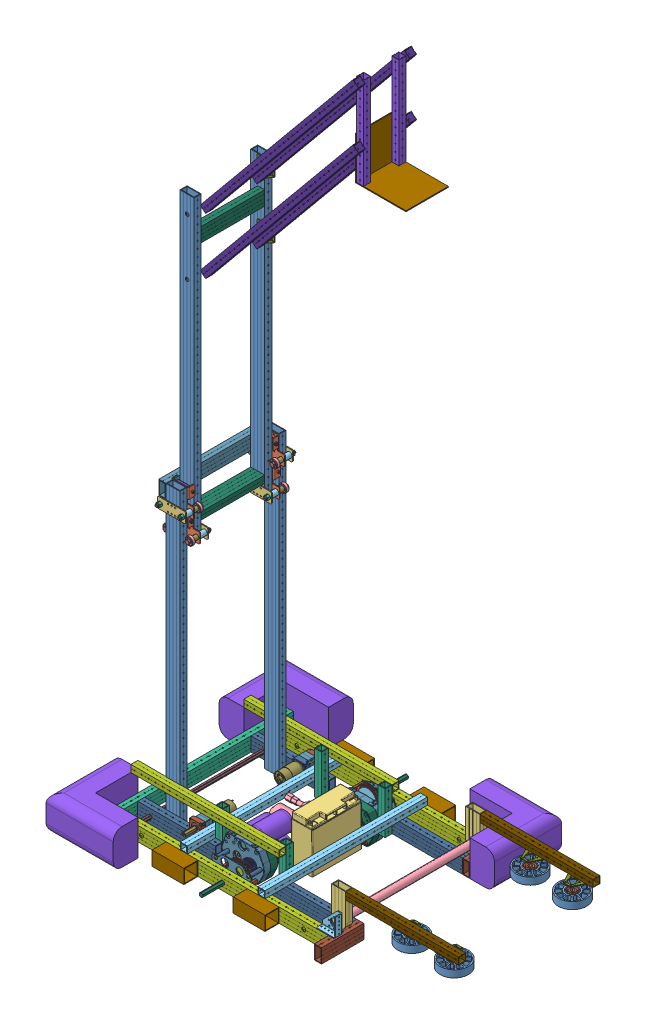
SolidWorks assembly Test Robot 2, configuration Default. Lengths in mm. (continued)
Components (placement in the parent): (continued)
- Test Base 2-1: Test Base 2 [Default] at (327.6786 481.923 -175.606) size (990.6 253.34 863.6) (continued)
  - 3 CIM Ball Shifter with WCD Output-2: 3 CIM Ball Shifter with WCD Output [Default] at (711.3612 320.9643 338.8075) x (0 -1 0) z (0 0 -1) size (169.11 183.68 312.65) (continued)
    - Nylock Nut_NNY2520-ZC-2: Nylock Nut_NNY2520-ZC [Default] at (48.8823 -3.175 37.846) x (0 0 -1) z (-1 0 0) size (12.85 11.89 7.62)
    - Nylock Nut_NNY2520-ZC-3: Nylock Nut_NNY2520-ZC [Default] at (44.45 85.725 7.8613) x (0 1 0) z (0 0 -1) size (12.85 11.89 7.62)
    - 276-1027-001-1: 276-1027-001 [Default] at (47.625 58.1787 6.35) x (0 1 0) z (-1 0 0) size (8.61 5.64 9.94)
    - 276-1027-001-2: 276-1027-001 [Default] at (-47.625 58.1787 6.35) x (0 -1 0) z (1 0 0) size (8.61 5.64 9.94)
    - SCREW-832-1750-1: SCREW-832-1750 [Default] at (-47.625 58.1787 47.0408) x (0 0 -1) z (-0.960822 -0.277167 0) size (46.66 7.92 7.92)
    - SCREW-832-1750-2: SCREW-832-1750 [Default] at (47.625 58.1787 47.0408) x (0 0 -1) z (-0.960822 -0.277167 0) size (46.66 7.92 7.92)
    - Nylock Nut_NNY2520-ZC-4: Nylock Nut_NNY2520-ZC [Default] at (44.45 -15.875 7.8613) x (0 1 0) z (0 0 -1) size (12.85 11.89 7.62)
    - 217-2428-004 Rev3-1: 217-2428-004 Rev3 [Default] at (0 53.4162 22.7711) x (-0.709585 0.70462 0) z (0 0 1) size (11 9.53 43.92)
    - SBS1_SBS-2520-1625SS-1: SBS1_SBS-2520-1625SS [Default] at (44.45 85.725 42.4688) x (0 0 -1) z (-0.251219 0.96793 0) size (45.3 11.2 11.18)
    - SBS1_SBS-2520-1625SS-2: SBS1_SBS-2520-1625SS [Default] at (44.45 -15.875 42.4688) x (0 0 -1) z (-0.251219 0.96793 0) size (45.3 11.2 11.18)
    - SBS1_SBS2520-1750-1: SBS1_SBS2520-1750 [Default] at (-44.45 85.725 7.4422) x (0 0 1) z (-0.031478 0.999504 0) size (48.48 11.22 11.17)
    - SBS1_SBS2520-1750-2: SBS1_SBS2520-1750 [Default] at (-44.45 -15.875 7.4422) x (0 0 1) z (-0.937114 -0.349025 0) size (48.48 11.22 11.17)
    - 217-2428-021 Rev1-1: 217-2428-021 Rev1 [Default] at (0 53.4162 9.5123) x (0.451333 -0.892356 0) z (0 0 1) size (15.88 15.88 3.17)
    - 217-2428-029 Rev1-1: 217-2428-029 Rev1 [Default] at (0 53.4162 36.957) x (0.999846 0.017557 0) z (0 0 1) size (15.88 15.88 1.12)
    - Grayhill Lock Washer-1: Grayhill Lock Washer [Default] at (12.7 -21.997 -18.6817) x (0.467173 -0.884166 0) z (0 0 1) size (19.69 19.69 0.74)
    - Grayhill Nut-1: Grayhill Nut [Default] at (12.7 -21.997 -17.0434) x (0.984088 0.177684 0) z (0 0 1) size (18.33 15.88 2.54)
    - 217-2000-1: 217-2000 [Default] at (0 92.8624 0) x (0 0 -1) z (0.223996 -0.97459 0) size (150.2 64.01 64.01)
    - 217-2000-2: 217-2000 [Default] at (-36.9798 39.6868 0) x (0 0 -1) z (0.996195 -0.087156 0) size (150.2 64.01 64.01)
    - 217-2000-3: 217-2000 [Default] at (36.9798 39.6868 0) x (0 0 -1) z (0.996195 0.087156 0) size (150.2 64.01 64.01)
    - Grahill Encoder-1: Grahill Encoder [Default] at (12.7 -21.997 -16.1798) x (-0.580071 0.814566 0) z (-0.814566 -0.580071 0) size (31.75 31.12 31.75)
    - 217-3195-009 Rev1_wcd 2-1: 217-3195-009 Rev1_wcd 2 [Default] at (0 85.725 50.546) x (-0.998427 -0.056065 0) z (0 0 1) size (12.7 12.7 41.27)
    - 217-3195-006 Rev1_WCD-1: 217-3195-006 Rev1_WCD [Default] at (-44.45 85.725 44.1452) x (0.5 0.866025 0) z (0 0 1) size (12.7 14.66 47.62)
    - 217-3195-009 Rev1_wcd 2-2: 217-3195-009 Rev1_wcd 2 [Default] at (0 -31.75 50.546) x (0.947633 0.319361 0) z (0 0 1) size (12.7 12.7 41.27)
    - 217-3195-006 Rev1_WCD-2: 217-3195-006 Rev1_WCD [Default] at (-44.45 -15.875 44.1452) x (0.5 -0.866025 0) z (0 0 1) size (12.7 14.66 47.62)
    - Nylock Nut_NNY2520-ZC-5: Nylock Nut_NNY2520-ZC [Default] at (0 -31.75 45.0723) x (-0.5 0.866025 0) z (0 0 -1) size (12.85 11.89 7.62)
    - Nylock Nut_NNY2520-ZC-6: Nylock Nut_NNY2520-ZC [Default] at (0 85.725 45.0723) x (-0.5 0.866025 0) z (0 0 -1) size (12.85 11.89 7.62)
    - SBS1_SBS-2520-2250-1: SBS1_SBS-2520-2250 [Default] at (0 -31.75 98.298) x (0 0 -1) z (-0.933488 -0.358607 0) size (61.18 11.22 11.17)
    - SBS1_SBS2520-0625ZC-1: SBS1_SBS2520-0625ZC [Default] at (-44.45 85.725 98.298) x (0 0 -1) z (0.400817 0.916158 0) size (19.57 11.22 11.17)
    - SBS1_SBS2520-0625ZC-2: SBS1_SBS2520-0625ZC [Default] at (-44.45 -15.875 98.298) x (0 0 -1) z (-0.75178 -0.659414 0) size (19.57 11.22 11.17)
    - SBS1_SBS-2520-2250-2: SBS1_SBS-2520-2250 [Default] at (0 85.725 98.298) x (0 0 -1) z (0.056677 -0.998393 0) size (61.18 11.22 11.17)
    - 217-3195-003 rev2-1: 217-3195-003 rev2 [Default] at (0 0 94.9452) size (88.62 139.7 3.17)
    - 217-2617-003 Rev1-1: 217-2617-003 Rev1 [Default] at (-39.878 35.5392 121.8535) x (-0.5 -0.866025 0) z (0 0 1) size (14.66 12.7 152.4)
    - 217-3109-001 Rev1-1: 217-3109-001 Rev1 [Default] at (-39.878 35.5392 49.1808) x (0 0 1) z (0.312889 -0.94979 0) size (7.94 28.57 28.57)
    - 217-2734-001 Rev3-1: 217-2734-001 Rev3 [Default] at (-39.878 35.5392 98.1202) x (1 0 0) z (0 1 0) size (31.12 7.94 31.12)
    - 217-2617-004 Rev1_97431A340_grv-1: 217-2617-004 Rev1_97431A340_grv [Default] at (-39.878 35.5392 54.8961) x (0 0 1) z (-0.124043 -0.992277 0) size (1.07 20.42 18.58)
    - 217-2617-004 Rev1_97431A340_grv-2: 217-2617-004 Rev1_97431A340_grv [Default] at (0 0 69.215) x (0 0 1) z (-0.124043 -0.992277 0) size (1.07 20.42 18.58)
    - 217-2702-001_20t-1: 217-2702-001_20t [Default] at (0 0 62.357) x (0.998435 0.055929 0) z (0 0 1) size (28.2 28.2 12.65)
    - 217-2715-002 Rev1_64t-1: 217-2715-002 Rev1_64t [Default] at (-39.878 35.5392 61.7541) x (0.866025 -0.5 0) z (0 0 1) size (84.3 84.3 12.65)
    - 217-2704-001_24-1: 217-2704-001_24 [Default] at (0 0 62.357) x (0.450781 0.892635 0) z (0 0 -1) size (33.29 33.29 12.65)
    - 217-2714-002 Rev1_60t-1: 217-2714-002 Rev1_60t [Default] at (-39.878 35.5392 61.7541) x (0.866025 -0.5 0) z (0 0 1) size (78.95 78.95 12.65)
    - 217-3221-002 Rev1-1: 217-3221-002 Rev1 [Default] at (-39.878 35.5392 61.7414) x (0 -1 0) z (0 0 1) size (71.39 71.45 12.62)
    - 217-2705-001_30t-1: 217-2705-001_30t [Default] at (0 0 62.357) x (0.547654 -0.836705 0) z (0 0 1) size (41.01 41.12 12.65)
    - 217-2712-002 Rev1_50t-1: 217-2712-002 Rev1_50t [Default] at (-39.878 35.5392 61.7541) x (0.866025 -0.5 0) z (0 0 1) size (66.7 66.76 12.65)
    - 217-2706-001_34t-1: 217-2706-001_34t [Default] at (0 0 62.357) x (0.998435 0.055929 0) z (0 0 1) size (46.46 46.56 12.65)
    - 217-3288-001 Rev3-1: 217-3288-001 Rev3 [Default] at (0 0 0.0889) x (0.055929 -0.998435 0) z (0 0 1) size (99.51 99.53 98.3)
      - 217-2428-008 Rev2-1: 217-2428-008 Rev2 [Default] at (0 0 10.2679) size (31.75 31.75 1.59)
      - 217-2428-028 Rev1_97633A250-1: 217-2428-028 Rev1_97633A250 [Default] at (0 0 37.1221) x (0 0 1) z (0.9357 -0.352797 0) size (1.07 23.39 21.18)
      - 217-4099-000 Rev2_high gear-1: 217-4099-000 Rev2_high gear [Default] x (-1 0 0) z (0 0 1) size (22.23 22.23 98.3)
        - 217-4098-005 Rev1_91612A226-1: 217-4098-005 Rev1_91612A226 [Default] at (0 0 46.2661) x (-0.144757 0 0.989467) z (0 -1 0) size (3.02 3.15 18.22)
        - 217-4098-003 Rev2-1: 217-4098-003 Rev2 [Default] x (1 0 0) z (0 0 -1) size (22.23 22.23 55.94)
        - 217-4099-002 Rev3-1: 217-4099-002 Rev3 [Default] at (0 0 53.467) x (0 0 1) z (-1 0 0) size (40.96 12.73 14.67)
        - 217-4098-004 Rev1-1: 217-4098-004 Rev1 [Default] at (0 0 14.2494) x (0.393904 0.919152 0) z (0 0 1) size (11.68 11.68 56)
      - 217-2428-007 Rev1-1: 217-2428-007 Rev1 [Default] at (7.809 4.5085 14.2494) x (-0.69071 0.455693 -0.561483) z (-0.67559 -0.683536 0.276329) size (6.35 6.35 6.35)
      - 217-2428-007 Rev1-2: 217-2428-007 Rev1 [Default] at (5.4343 3.1375 26.9494) x (-0.162331 -0.978398 0.128005) z (0.857281 -0.204076 -0.472676) size (6.35 6.35 6.35)
      - 217-3212-101 Rev1-1: 217-3212-101 Rev1 [Default] at (-11.5751 10.4131 45.3224) x (0.923728 0.383049 0) z (0 0 -1) size (46.46 46.56 12.7)
        - 217-2428-022 Rev1-1: 217-2428-022 Rev1 [Default] at (6.7035 14.0527 24.6087) size (28.57 28.57 6.1)
        - 217-3212-001 Rev1_34t-1: 217-3212-001 Rev1_34t [Default] at (6.7035 14.0527 27.9107) size (46.46 46.56 11.11)
      - 217-3222-101 Rev1-1: 217-3222-101 Rev1 [Default] at (21.0941 -5.2804 52.7371) x (-0.889163 -0.457591 0) z (0 0 -1) size (73.87 73.92 12.7)
        - 217-2428-022 Rev1-1: 217-2428-022 Rev1 [Default] at (16.3398 14.3476 19.3234) size (28.57 28.57 6.1)
        - 217-3222-001 Rev1_Spur01-1: 217-3222-001 Rev1_Spur01 [Default] at (16.3398 14.3476 22.6254) x (0.999377 0.0353 0) z (0 0 1) size (71.39 71.45 11.11)
      - 217-2428-007 Rev1-3: 217-2428-007 Rev1 [Default] at (-5.4343 3.1375 26.9494) x (0.928483 0.348617 0.128005) z (-0.251905 0.844465 -0.472676) size (6.35 6.35 6.35)
      - 217-2428-007 Rev1-4: 217-2428-007 Rev1 [Default] at (0 -6.275 26.9494) x (-0.766153 0.629782 0.128005) z (-0.605376 -0.640389 -0.472676) size (6.35 6.35 6.35)
      - 217-2428-007 Rev1-5: 217-2428-007 Rev1 [Default] at (-7.809 4.5085 14.2494) x (-0.049287 -0.826019 -0.561483) z (0.929754 -0.24331 0.276329) size (6.35 6.35 6.35)
      - 217-2428-007 Rev1-6: 217-2428-007 Rev1 [Default] at (0 -9.017 14.2494) x (0.739997 0.370326 -0.561483) z (-0.254164 0.926846 0.276329) size (6.35 6.35 6.35)
    - 217-3210-001 Rev1_30t-1: 217-3210-001 Rev1_30t [Default] at (0 53.4162 30.0736) x (-0.966828 0.255427 0) z (0 0 1) size (41.01 41.12 12.65)
    - 217-2711-002 Rev1_50t-1: 217-2711-002 Rev1_50t [Default] at (0 53.4162 17.4244) x (0.262208 -0.965011 0) z (0 0 1) size (66.7 66.76 12.65)
  - Base Front Rail-2: Base Front Rail [Default] at (1069.5219 360.9185 -429.2377) size (25.4 50.8 152.4)
  - Blue Bumper-3: Blue Bumper [Default] at (180.5219 335.5185 942.3623) size (241.3 127 241.3)
  - Blue Bumper-4: Blue Bumper [Default] at (180.5219 335.5185 78.7623) x (0 0 1) z (-1 0 0) size (241.3 127 241.3)
  - Battery_12V-1: Battery_12V [Default] at (781.3061 335.5185 454.7754) x (0 0 1) z (0 1 0) size (177.8 76.2 167.13)
  - Compressor_90C-1: Compressor_90C [Default] at (627.7537 373.1105 499.1323) x (0 0 -1) z (1 0 0) size (53.59 121.98 156.21)
  - Base Side Rail Internal-5: Base Side Rail Internal [Default] at (307.5219 360.9185 307.3623) x (0 0 -1) z (1 0 0) size (25.4 50.8 279.4)
  - Base Side Rail Internal-6: Base Side Rail Internal [Default] at (307.5219 360.9185 713.7623) x (0 0 -1) z (1 0 0) size (25.4 50.8 279.4)
  - Superstructure Lower Crossbar-1: Superstructure Lower Crossbar [Default] at (815.5219 399.0185 53.3623) size (25.4 25.4 584.2)
  - Superstructure Upright-1: Superstructure Upright [Default] at (790.1219 1084.8185 688.3623) x (1 0 0) z (0 -1 0) size (25.4 25.4 152.4)
  - Superstructure Upright-2: Superstructure Upright [Default] at (790.1219 1084.8185 332.7623) x (1 0 0) z (0 -1 0) size (25.4 25.4 152.4)
  - Superstructure Upright-3: Superstructure Upright [Default] at (561.5219 1084.8185 332.7623) x (1 0 0) z (0 -1 0) size (25.4 25.4 152.4)
  - Superstructure Upright-4: Superstructure Upright [Default] at (561.5219 1084.8185 689.3363) x (1 0 0) z (0 -1 0) size (25.4 25.4 152.4)
  - Superstructure Lower Crossbar-2: Superstructure Lower Crossbar [Default] at (536.1219 399.0185 53.3623) size (25.4 25.4 584.2)
  - Superstructure Crossbar-1: Superstructure Crossbar [Default] at (53.5219 475.2185 713.7623) x (0 0 -1) z (1 0 0) size (25.4 25.4 533.4)
  - Superstructure Crossbar-2: Superstructure Crossbar [Default] at (53.5219 475.2185 307.3623) x (0 0 -1) z (1 0 0) size (25.4 25.4 533.4)
- PowerUp Cube-3: PowerUp Cube [Default] at (1484.2166 1060.7016 182.5563) x (1 0 0) z (0 0 -1) size (330.2 279.4 330.2) (hidden)
- Intake Mechansim-1: Intake Mechansim [Default] at (1364.1836 3104.9251 338.871) x (-1 0 0) z (0 1 0) size (25.4 25.4 330.2)
  - Elevator Top Crossbar-1: Elevator Top Crossbar [Default] at (81.2508 124.0592 -460.6133) size (25.4 25.4 330.2) (hidden)
- PowerUp Cube-4: PowerUp Cube [Default] at (1295.6328 3203.1118 170.8303) x (1 0 0) z (0 0 -1) size (330.2 279.4 330.2) (hidden)
- VersaFrame Corner Gusset-2: VersaFrame Corner Gusset [Default] at (1409.9006 868.2415 601.6563) x (0 1 0) z (0 0 1) size (69.72 69.72 25.4)
- Top Bottom Grasper-1: Top Bottom Grasper [Default] at (1103.9738 3449.2709 552.0299) x (0 0 -1) z (0 -1 0) size (152.4 180.97 333.38)
  - Elevator Top Crossbar-1: Elevator Top Crossbar [Default] at (152.5996 178.9591 -350.7409) size (25.4 25.4 330.2)
  - Elevator Top Crossbar-2: Elevator Top Crossbar [Default] at (279.5996 178.9591 -350.7409) size (25.4 25.4 330.2)
  - Cube Intake Bottom Support-1: Cube Intake Bottom Support [Default] at (139.8996 163.0841 246.1591) x (0 1 0) z (1 0 0) size (180.97 155.57 152.4)
- 217-2 Stage Versaplanetary STEP-1: 217-2 Stage Versaplanetary STEP [Default] at (830.1006 889.2415 170.5813) size (44.3 44.3 179.1)
  - 217-2625-001 Rev1-1: 217-2625-001 Rev1 [Default] at origin size (42 42 18)
  - 217-2625-002 Rev1-1: 217-2625-002 Rev1 [Default] at (0 0 -29.4) size (42 42 17.13)
  - 217-2625-003 Rev1-1: 217-2625-003 Rev1 [Default] at (0 0 -43.6478) x (1 0 0) z (0 0 -1) size (17 17 64.12)
  - 217-2625-009 Rev1-1: 217-2625-009 Rev1 [Default] at (0 0 -3.48) x (0 -1 0) z (0 0 -1) size (18 18 13)
  - 217-2816-001 Rev1-1: 217-2816-001 Rev1 [Default] at (0 0 -16.85) x (1 0 0) z (0 0 -1) size (42 42 14.5)
  - 217-2625-007 Rev1_Sun_Driver01-1: 217-2625-007 Rev1_Sun_Driver01 [Default] at (0 0 -11.767) x (0.055822 0.998441 0) z (0 0 1) size (14.49 14.49 12.72)
  - 217-2625-100-1: 217-2625-100 [Default] at (0 0 -18.467) x (0 1 0) z (0 0 1) size (39.26 38.9 12.7)
    - 217-2625-008 Rev1-1: 217-2625-008 Rev1 [Default] at origin size (34.7 34.7 4.7)
    - 217-2625-010 Rev1-1: 217-2625-010 Rev1 [Default] at (0 10.193 3.65) x (0.999813 0.019336 0) z (0 0 1) size (4 4 12)
    - 217-2625-010 Rev1-2: 217-2625-010 Rev1 [Default] at (8.691 -5.3258 3.65) size (4 4 12)
    - 217-2625-010 Rev1-3: 217-2625-010 Rev1 [Default] at (-8.691 -5.3258 3.65) size (4 4 12)
    - 217-2625-005 Rev1_Planet_Revolving_Follower01-1: 217-2625-005 Rev1_Planet_Revolving_Follower01 [Default] at (8.691 -5.3258 6.35) x (0.932816 0.360354 0) z (0 0 1) size (16.91 16.92 8)
    - 217-2625-005 Rev1_Planet_Revolving_Follower01-2: 217-2625-005 Rev1_Planet_Revolving_Follower01 [Default] at (-8.691 -5.3258 6.35) x (-0.932788 -0.360426 0) z (0 0 1) size (16.91 16.92 8)
    - 217-2625-005 Rev1_Planet_Revolving_Follower01-3: 217-2625-005 Rev1_Planet_Revolving_Follower01 [Default] at (0 10.193 6.35) x (0.893583 0.448898 0) z (0 0 1) size (16.91 16.92 8)
  - 217-2822-003 Rev4-1: 217-2822-003 Rev4 [Default] at (0 0 9) x (0 1 0) z (0 0 1) size (42 42 4.8)
  - 217-2625-011 Rev1-1: 217-2625-011 Rev1 [Default] at (0 0 1.37) x (1 0 0) z (0 -1 0) size (8.01 7.5 7.94)
  - SSA_SSA0832-0500ZC-1: SSA_SSA0832-0500ZC [Default] at (17.5 -17.5 10.5) x (0.189399 -0.9819 0) z (-0.9819 -0.189399 0) size (6.73 16.76 6.73)
  - 217-2742-1: 217-2742 [Default] at (0 0 -43.1002) x (0 0 1) z (-1 0 0) size (7 28 28)
  - 217-2742-2: 217-2742 [Default] at (0 0 -51.4002) x (0 0 1) z (-0.997393 0.072165 0) size (7 28 28)
  - SSA_SSA0832-1750ZC-1: SSA_SSA0832-1750ZC [Default] at (17.5 -17.5 -47.261) x (1 0 0) z (0 1 0) size (6.73 48.51 6.73)
  - SSA_SSA0832-1750ZC-2: SSA_SSA0832-1750ZC [Default] at (-17.5 17.5 -47.261) x (1 0 0) z (0 1 0) size (6.73 48.51 6.73)
  - 217-2625-018 Rev1_98541A410-1: 217-2625-018 Rev1_98541A410 [Default] at (0 0 -35.4954) x (0 0 -1) z (0.980859 -0.194721 0) size (1 19.6 17.4)
  - 217-2625-017 Rev1_9714K61-1: 217-2625-017 Rev1_9714K61 [Default] at (0 0 -44.1002) x (-0.695225 0.718792 0) z (-0.718792 -0.695225 0) size (28.51 4.98 30.18)
  - PINL-M020-006-S-1: PINL-M020-006-S [Default] at (-18.5 13.6657 -9.5) x (0 0 -1) z (1 0 0) size (6 2 2)
  - PINL-M020-006-S-2: PINL-M020-006-S [Default] at (-18.5 13.6657 -22.2) x (0 0 -1) z (0.23951 -0.970894 0) size (6 2 2)
  - 217-2816-001 Rev1-2: 217-2816-001 Rev1 [Default] at (0 0 -29.55) x (1 0 0) z (0 0 -1) size (42 42 14.5)
  - 217-3106-000 Rev2_NO SUN-1: 217-3106-000 Rev2_NO SUN [Default] at (0 0 -31.5454) size (40.34 37.58 17.71)
    - 217-3106-002 Rev1_Planet_Revolving_Follower01-1: 217-3106-002 Rev1_Planet_Revolving_Follower01 [Default] at (0 10.2965 6.35) x (0.979503 -0.20143 0) z (0 0 1) size (16.8 16.83 8)
    - 217-3106-003 Rev1-1: 217-3106-003 Rev1 [Default] at origin size (34.7 34.7 4.7)
    - 217-3106-001 Rev1_Sun_Driver01-1: 217-3106-001 Rev1_Sun_Driver01 [Default] at (0 0 9.0125) x (1 0 0) z (0 0 -1) size (14.56 14.56 12.7)
    - 217-3106-002 Rev1_Planet_Revolving_Follower01-2: 217-3106-002 Rev1_Planet_Revolving_Follower01 [Default] at (8.917 -5.1482 6.35) x (-0.664195 -0.74756 0) z (0 0 1) size (16.8 16.83 8)
    - 217-3106-002 Rev1_Planet_Revolving_Follower01-3: 217-3106-002 Rev1_Planet_Revolving_Follower01 [Default] at (-8.917 -5.1482 6.35) x (-0.315308 0.948989 0) z (0 0 1) size (16.8 16.83 8)
    - 217-2625-010 Rev1-1: 217-2625-010 Rev1 [Default] at (8.917 -5.1482 3.65) x (0.999617 0.027658 0) z (0 0 1) size (4 4 12)
    - 217-2625-010 Rev1-2: 217-2625-010 Rev1 [Default] at (-8.917 -5.1482 3.65) x (-0.475856 -0.879523 0) z (0 0 1) size (4 4 12)
    - 217-2625-010 Rev1-3: 217-2625-010 Rev1 [Default] at (0 10.2965 3.65) x (-0.523761 0.851865 0) z (0 0 1) size (4 4 12)
  - 775 pro-1: 775 pro [Default] at (0 0 10.5) x (0 0 1) z (-1 0 0) size (88 44.3 44.3)
- 217-2 Stage Versaplanetary STEP-2: 217-2 Stage Versaplanetary STEP [Default] at (830.1006 889.2415 500.3053) x (-1 0 0) z (0 0 -1) size (44.3 44.3 179.1)
  - 217-2625-001 Rev1-1: 217-2625-001 Rev1 [Default] at origin size (42 42 18)
  - 217-2625-002 Rev1-1: 217-2625-002 Rev1 [Default] at (0 0 -29.4) size (42 42 17.13)
  - 217-2625-003 Rev1-1: 217-2625-003 Rev1 [Default] at (0 0 -43.6478) x (1 0 0) z (0 0 -1) size (17 17 64.12)
  - 217-2625-009 Rev1-1: 217-2625-009 Rev1 [Default] at (0 0 -3.48) x (0 -1 0) z (0 0 -1) size (18 18 13)
  - 217-2816-001 Rev1-1: 217-2816-001 Rev1 [Default] at (0 0 -16.85) x (1 0 0) z (0 0 -1) size (42 42 14.5)
  - 217-2625-007 Rev1_Sun_Driver01-1: 217-2625-007 Rev1_Sun_Driver01 [Default] at (0 0 -11.767) x (0.055822 0.998441 0) z (0 0 1) size (14.49 14.49 12.72)
  - 217-2625-100-1: 217-2625-100 [Default] at (0 0 -18.467) x (0 1 0) z (0 0 1) size (39.26 38.9 12.7)
    - 217-2625-008 Rev1-1: 217-2625-008 Rev1 [Default] at origin size (34.7 34.7 4.7)
    - 217-2625-010 Rev1-1: 217-2625-010 Rev1 [Default] at (0 10.193 3.65) x (0.999813 0.019336 0) z (0 0 1) size (4 4 12)
    - 217-2625-010 Rev1-2: 217-2625-010 Rev1 [Default] at (8.691 -5.3258 3.65) size (4 4 12)
    - 217-2625-010 Rev1-3: 217-2625-010 Rev1 [Default] at (-8.691 -5.3258 3.65) size (4 4 12)
    - 217-2625-005 Rev1_Planet_Revolving_Follower01-1: 217-2625-005 Rev1_Planet_Revolving_Follower01 [Default] at (8.691 -5.3258 6.35) x (0.932816 0.360354 0) z (0 0 1) size (16.91 16.92 8)
    - 217-2625-005 Rev1_Planet_Revolving_Follower01-2: 217-2625-005 Rev1_Planet_Revolving_Follower01 [Default] at (-8.691 -5.3258 6.35) x (-0.932788 -0.360426 0) z (0 0 1) size (16.91 16.92 8)
    - 217-2625-005 Rev1_Planet_Revolving_Follower01-3: 217-2625-005 Rev1_Planet_Revolving_Follower01 [Default] at (0 10.193 6.35) x (0.893583 0.448898 0) z (0 0 1) size (16.91 16.92 8)
  - 217-2822-003 Rev4-1: 217-2822-003 Rev4 [Default] at (0 0 9) x (0 1 0) z (0 0 1) size (42 42 4.8)
  - 217-2625-011 Rev1-1: 217-2625-011 Rev1 [Default] at (0 0 1.37) x (1 0 0) z (0 -1 0) size (8.01 7.5 7.94)
  - SSA_SSA0832-0500ZC-1: SSA_SSA0832-0500ZC [Default] at (17.5 -17.5 10.5) x (0.189399 -0.9819 0) z (-0.9819 -0.189399 0) size (6.73 16.76 6.73)
  - 217-2742-1: 217-2742 [Default] at (0 0 -43.1002) x (0 0 1) z (-1 0 0) size (7 28 28)
  - 217-2742-2: 217-2742 [Default] at (0 0 -51.4002) x (0 0 1) z (-0.997393 0.072165 0) size (7 28 28)
  - SSA_SSA0832-1750ZC-1: SSA_SSA0832-1750ZC [Default] at (17.5 -17.5 -47.261) x (1 0 0) z (0 1 0) size (6.73 48.51 6.73)
  - SSA_SSA0832-1750ZC-2: SSA_SSA0832-1750ZC [Default] at (-17.5 17.5 -47.261) x (1 0 0) z (0 1 0) size (6.73 48.51 6.73)
  - 217-2625-018 Rev1_98541A410-1: 217-2625-018 Rev1_98541A410 [Default] at (0 0 -35.4954) x (0 0 -1) z (0.980859 -0.194721 0) size (1 19.6 17.4)
  - 217-2625-017 Rev1_9714K61-1: 217-2625-017 Rev1_9714K61 [Default] at (0 0 -44.1002) x (-0.695225 0.718792 0) z (-0.718792 -0.695225 0) size (28.51 4.98 30.18)
  - PINL-M020-006-S-1: PINL-M020-006-S [Default] at (-18.5 13.6657 -9.5) x (0 0 -1) z (1 0 0) size (6 2 2)
  - PINL-M020-006-S-2: PINL-M020-006-S [Default] at (-18.5 13.6657 -22.2) x (0 0 -1) z (0.23951 -0.970894 0) size (6 2 2)
  - 217-2816-001 Rev1-2: 217-2816-001 Rev1 [Default] at (0 0 -29.55) x (1 0 0) z (0 0 -1) size (42 42 14.5)
  - 217-3106-000 Rev2_NO SUN-1: 217-3106-000 Rev2_NO SUN [Default] at (0 0 -31.5454) size (40.34 37.58 17.71)
    - 217-3106-002 Rev1_Planet_Revolving_Follower01-1: 217-3106-002 Rev1_Planet_Revolving_Follower01 [Default] at (0 10.2965 6.35) x (0.979503 -0.20143 0) z (0 0 1) size (16.8 16.83 8)
    - 217-3106-003 Rev1-1: 217-3106-003 Rev1 [Default] at origin size (34.7 34.7 4.7)
    - 217-3106-001 Rev1_Sun_Driver01-1: 217-3106-001 Rev1_Sun_Driver01 [Default] at (0 0 9.0125) x (1 0 0) z (0 0 -1) size (14.56 14.56 12.7)
    - 217-3106-002 Rev1_Planet_Revolving_Follower01-2: 217-3106-002 Rev1_Planet_Revolving_Follower01 [Default] at (8.917 -5.1482 6.35) x (-0.664195 -0.74756 0) z (0 0 1) size (16.8 16.83 8)
    - 217-3106-002 Rev1_Planet_Revolving_Follower01-3: 217-3106-002 Rev1_Planet_Revolving_Follower01 [Default] at (-8.917 -5.1482 6.35) x (-0.315308 0.948989 0) z (0 0 1) size (16.8 16.83 8)
    - 217-2625-010 Rev1-1: 217-2625-010 Rev1 [Default] at (8.917 -5.1482 3.65) x (0.999617 0.027658 0) z (0 0 1) size (4 4 12)
    - 217-2625-010 Rev1-2: 217-2625-010 Rev1 [Default] at (-8.917 -5.1482 3.65) x (-0.475856 -0.879523 0) z (0 0 1) size (4 4 12)
    - 217-2625-010 Rev1-3: 217-2625-010 Rev1 [Default] at (0 10.2965 3.65) x (-0.523761 0.851865 0) z (0 0 1) size (4 4 12)
  - 775 pro-1: 775 pro [Default] at (0 0 10.5) x (0 0 1) z (-1 0 0) size (88 44.3 44.3)
- Elevator Hex Shaft-1: Elevator Hex Shaft [Default] at (667.4706 842.8161 144.4563) size (13.74 12.75 533.4)
Mates (geometry in assembly coordinates):
- Distance6: distance = 25.4 mm anti-aligned: plane of Elevator Moving Stage-1/Elevator Fixed Frame-1 through (749.5006 2773.2415 196.2303) normal (0 0 -1); plane of Elevator Base Frame-1/Elevator Fixed Frame-2 through (698.7006 1884.2415 170.8303) normal (0 0 1)
- Coincident11: coincident aligned: plane of Elevator Base Frame-1/Elevator Fixed Frame-1 through (749.5006 1884.2415 501.0303) normal (1 0 0); plane of Elevator Moving Stage-1/Elevator Fixed Frame-2 through (749.5006 2773.2415 475.6303) normal (1 0 0)
- LimitDistance1: limit distance = 889 mm aligned: plane of Elevator Base Frame-1/Elevator Fixed Frame-1 through (724.1006 1884.2415 513.7303) normal (0 1 0); plane of Elevator Moving Stage-1/Elevator Fixed Frame-2 through (724.1006 2773.2415 462.9303) normal (0 1 0)
- Distance11: distance = 6.35 mm anti-aligned: plane of Elevator Moving Stage-1/Elevator Fixed Frame-2 through (749.5006 2773.2415 450.2303) normal (0 0 -1); plane of Elevator Arm Section-1 through (758.9944 2510.6197 443.8803) normal (0 0 1)
- Coincident20: coincident aligned: plane of Elevator Arm Section-1 through (758.9944 2510.6197 443.8803) normal (0 0 1); plane of Elevator Arm Section-2 through (758.9944 2713.8197 443.8803) normal (0 0 1)
- Angle3: planar angle = 0 rad aligned: plane of Elevator Arm Section-1 through (739.4094 2526.7933 443.8803) normal (-0.771063 0.636758 0); plane of Elevator Arm Section-2 through (739.4094 2729.9933 443.8803) normal (-0.771063 0.636758 0)
- LimitAngle3: limit planar angle = 1.047198 rad aligned: plane of Elevator Arm Section-2; plane of ? through (-190.1651 1443.1853 1131.7973) normal (0 1 0)
- Coincident30: coincident anti-aligned: plane of ? through (698.7006 1960.4415 475.6303) normal (-1 0 0); plane of ? through (698.7006 1071.4415 869.3303) normal (1 0 0)
- Coincident31: coincident aligned: plane of Elevator Base Frame-1/Elevator Fixed Frame-1 through (698.7006 1884.2415 526.4303) normal (0 0 1); plane of Intake Mechanism-2/Intake Arm-2 through (608.7881 1138.2851 526.4303) normal (0 0 1)
- Distance25: distance = 76.2 mm: line of Elevator Moving Stage-1/Elevator Crossbar-1 through (711.3244 969.8415 221.6303) axis (0 0 1); plane of ? through (698.7006 1046.0415 120.0303) normal (0 -1 0)
- Coincident47: coincident anti-aligned: plane of Elevator Base Frame-1/Elevator Fixed Frame-1 through (698.7006 1884.2415 526.4303) normal (0 0 1); plane of Test Base 2-1/Base Side Rail Internal-4 through (622.5006 817.4415 526.4303) normal (0 0 -1)
- Coincident48: coincident aligned: plane of Elevator Base Frame-1/Elevator Fixed Frame-1 through (724.1006 817.4415 513.7303) normal (0 -1 0); plane of Test Base 2-1/Base Rear Rail-1 through (597.1006 817.4415 677.8563) normal (0 -1 0)
- Distance31: distance = 76.2 mm anti-aligned: plane of Elevator Base Frame-1/Elevator Fixed Frame-1 through (698.7006 1884.2415 501.0303) normal (-1 0 0); plane of Test Base 2-1/Base Rear Rail-1 through (622.5006 817.4415 677.8563) normal (1 0 0)
- Concentric6: concentric anti-aligned: cylinder of Elevator Moving Stage-1/VersaFrame Side Bearing Mount-1 through (765.3756 2741.4915 221.6303) axis (0 0 1) radius 14.2875; cylinder of Elevator Arm Section-2 through (765.3756 2741.4915 443.8803) axis (0 0 -1) radius 2.0701
- Distance34: distance = 57.15 mm anti-aligned: plane of Intake Mechansim-1/Elevator Top Crossbar-1 through (1295.6328 3393.6118 475.6303) normal (0 0 1); plane of Elevator Arm Section-2 through (758.9944 2713.8197 418.4803) normal (0 0 -1)
- Angle6: planar angle = 0 rad aligned: plane of Intake Mechansim-1/Elevator Top Crossbar-1 through (1295.6328 3393.6118 450.2303) normal (1 0 0); plane of Elevator Base Frame-1/Elevator Fixed Frame-1 through (749.5006 1884.2415 501.0303) normal (1 0 0)
- Concentric10: concentric anti-aligned: cylinder of Elevator Arm Section-2 through (1282.9328 3368.2118 443.8803) axis (0 0 -1) radius 2.0701; cylinder of Intake Mechansim-1/Elevator Top Crossbar-1 through (1282.9328 3368.2118 450.2303) axis (0 0 1) radius 2.0701
- Concentric11: concentric aligned: cylinder of Elevator Moving Stage-1/VersaFrame Side Bearing Mount-2 through (765.3756 2538.2915 221.6303) axis (0 0 1) radius 14.2875; circle of Elevator Arm Section-1
- Distance35: distance = 25.4 mm aligned: plane of PowerUp Cube-4 through (1295.6328 2923.7118 501.0303) normal (0 0 1); plane of Intake Mechansim-1/Elevator Top Crossbar-1 through (1295.6328 3393.6118 475.6303) normal (0 0 1)
- Distance36: distance = 0 mm anti-aligned: plane of Intake Mechansim-1/Elevator Top Crossbar-1 through (1295.6328 3393.6118 450.2303) normal (1 0 0); plane of PowerUp Cube-4 through (1295.6328 2923.7118 170.8303) normal (-1 0 0)
- Distance38: distance = 190.5 mm aligned: plane of PowerUp Cube-4 through (1295.6328 3203.1118 170.8303) normal (0 1 0); plane of Intake Mechansim-1/Elevator Top Crossbar-1 through (1282.9328 3393.6118 462.9303) normal (0 1 0)
- LimitAngle4: limit planar angle = 2.451306 rad aligned: plane of Elevator Arm Section-2 through (739.4094 2729.9933 443.8803) normal (-0.771063 0.636758 0); plane of Elevator Moving Stage-1/Elevator Fixed Frame-2 through (749.5006 2773.2415 475.6303) normal (1 0 0)
- Coincident50: coincident anti-aligned: plane of VersaFrame Corner Gusset-1 through (1409.9006 868.2415 68.2563) normal (0 -1 0); plane of Test Base 2-1/Base Side Rail Internal-5 through (1384.5006 868.2415 144.4563) normal (0 1 0)
- Coincident51: coincident anti-aligned: plane of VersaFrame Corner Gusset-1 through (1409.9006 868.2415 68.2563) normal (1 0 0); plane of Test Base 2-1/Blue Bumper-2 through (1409.9006 944.4415 -96.8437) normal (-1 0 0)
- Coincident53: coincident aligned: plane of VersaFrame Corner Gusset-1 through (1409.9006 868.2415 68.2563) normal (0 0 1); plane of Test Base 2-1/Base Side Rail-2 through (622.5006 817.4415 68.2563) normal (0 0 1)
- Distance40: distance = 12.7 mm anti-aligned: plane of VersaFrame Corner Gusset-1 through (1409.9006 868.2415 68.2563) normal (0 0 1); plane of Intake Mechanism-3/Intake Upright 2-1 through (1382.6166 1619.5016 80.9563) normal (0 0 -1)
- Concentric12: concentric aligned: cylinder of Intake Mechanism-3/Intake Upright 2-1 through (1382.5404 895.6016 80.9563) axis (0 0 1) radius 6.35; cylinder of VersaFrame Corner Gusset-1 through (1382.5404 895.6016 65.0813) axis (0 0 1) radius 14.2875
- Coincident54: coincident anti-aligned: plane of Test Base 2-1/Base Side Rail-1 through (622.5006 868.2415 601.6563) normal (0 1 0); plane of VersaFrame Corner Gusset-2 through (1409.9006 868.2415 601.6563) normal (0 -1 0)
- Coincident55: coincident anti-aligned: plane of Test Base 2-1/Blue Bumper-1 through (1409.9006 944.4415 766.7563) normal (-1 0 0); plane of VersaFrame Corner Gusset-2 through (1409.9006 868.2415 601.6563) normal (1 0 0)
- Coincident56: coincident aligned: plane of Test Base 2-1/Base Side Rail-1 through (622.5006 817.4415 601.6563) normal (0 0 -1); plane of VersaFrame Corner Gusset-2 through (1409.9006 868.2415 601.6563) normal (0 0 -1)
- Concentric13: concentric aligned: cylinder of Elevator Arm Section-2 through (1282.9328 3368.2118 443.8803) axis (0 0 -1) radius 2.0701; cylinder of Top Bottom Grasper-1/Elevator Top Crossbar-1 through (1282.9328 3368.2118 412.1303) axis (0 0 -1) radius 2.0701
- Distance43: distance = 6.35 mm anti-aligned: plane of Top Bottom Grasper-1/Elevator Top Crossbar-1 through (1270.2328 3050.7118 412.1303) normal (0 0 1); plane of Elevator Arm Section-2 through (758.9944 2713.8197 418.4803) normal (0 0 -1)
- Angle10: planar angle = 0 rad aligned: plane of Elevator Base Frame-1/Elevator Fixed Frame-1 through (749.5006 1884.2415 501.0303) normal (1 0 0); plane of Top Bottom Grasper-1/Elevator Top Crossbar-1 through (1295.6328 3050.7118 412.1303) normal (1 0 0)
- Concentric14: concentric aligned: cylinder of Elevator Moving Stage-1/VersaFrame Side Bearing Mount-1 through (765.3756 2741.4915 221.6303) axis (0 0 1) radius 14.2875; circle of Elevator Arm Section-3
- Angle11: planar angle = 0 rad aligned: plane of Elevator Arm Section-2 through (739.4094 2729.9933 443.8803) normal (-0.771063 0.636758 0); plane of Elevator Arm Section-3 through (739.4094 2729.9933 259.7303) normal (-0.771063 0.636758 0)
- Distance46: distance = 12.7 mm anti-aligned: plane of Elevator Arm Section-3 through (758.9944 2713.8197 234.3303) normal (0 0 -1); plane of Elevator Moving Stage-1/Elevator Fixed Frame-1 through (749.5006 2773.2415 221.6303) normal (0 0 1)
- Concentric15: concentric anti-aligned: cylinder of Elevator Moving Stage-1/VersaFrame Side Bearing Mount-2 through (765.3756 2538.2915 221.6303) axis (0 0 1) radius 14.2875; cylinder of Elevator Arm Section-4 through (765.3756 2538.2915 259.7303) axis (0 0 -1) radius 2.0701
- Angle12: planar angle = 0 rad aligned: plane of Elevator Arm Section-4 through (739.4094 2526.7933 259.7303) normal (-0.771063 0.636758 0); plane of Elevator Arm Section-3 through (739.4094 2729.9933 259.7303) normal (-0.771063 0.636758 0)
- Coincident59: coincident aligned: plane of Elevator Arm Section-3 through (758.9944 2713.8197 259.7303) normal (0 0 1); plane of Elevator Arm Section-4 through (758.9944 2510.6197 259.7303) normal (0 0 1)
- LimitAngle5: limit planar angle = 1.570796 rad aligned: plane of Test Base 2-1/Base Side Rail Internal-6 through (1384.5006 868.2415 550.8563) normal (0 1 0); plane of Intake Mechanism-3/Intake Upright 2-2 through (1408.0166 870.2016 563.5563) normal (1 0 0)
- Coincident60: coincident anti-aligned: plane of Test Base 2-1/Base Side Rail Internal-1 through (901.9006 868.2415 144.4563) normal (0 1 0); plane of 217-2 Stage Versaplanetary STEP-1/217-2625-002 Rev1-1 through (851.1006 868.2415 119.0563) normal (0 -1 0)
- Coincident61: coincident aligned: plane of Test Base 2-1/Base Side Rail Internal-1 through (901.9006 817.4415 119.0563) normal (0 0 -1); plane of 217-2 Stage Versaplanetary STEP-1/217-2625-002 Rev1-1 through (809.1006 910.2415 119.0563) normal (0 0 -1)
- Coincident62: coincident anti-aligned: plane of Test Base 2-1/Superstructure Lower Crossbar-2 through (851.1006 868.2415 627.0563) normal (-1 0 0); plane of 217-2 Stage Versaplanetary STEP-1/217-2625-002 Rev1-1 through (851.1006 868.2415 119.0563) normal (1 0 0)
- Coincident63: coincident anti-aligned: plane of Test Base 2-1/Base Side Rail Internal-4 through (622.5006 868.2415 526.4303) normal (0 1 0); plane of 217-2 Stage Versaplanetary STEP-2/217-2625-001 Rev1-1 through (851.1006 868.2415 504.3053) normal (0 -1 0)
- Coincident64: coincident aligned: plane of Test Base 2-1/Base Side Rail Internal-4 through (622.5006 817.4415 551.8303) normal (0 0 1); plane of 217-2 Stage Versaplanetary STEP-2/217-2625-002 Rev1-1 through (851.1006 910.2415 551.8303) normal (0 0 1)
- Coincident65: coincident anti-aligned: plane of Test Base 2-1/Superstructure Lower Crossbar-2 through (851.1006 868.2415 627.0563) normal (-1 0 0); plane of 217-2 Stage Versaplanetary STEP-2/217-2625-002 Rev1-1 through (851.1006 868.2415 551.8303) normal (1 0 0)
- Distance47: distance = 19.05 mm aligned: plane of Elevator Hex Shaft-1 through (671.1514 849.1915 601.6563) normal (0 1 0); plane of Test Base 2-1/Base Side Rail Internal-1 through (901.9006 868.2415 144.4563) normal (0 1 0)
- Distance48: distance = 50.8 mm aligned: plane of Test Base 2-1/Base Side Rail Internal-1 through (901.9006 817.4415 119.0563) normal (0 0 -1); plane of Elevator Hex Shaft-1 through (667.4706 842.8161 68.2563) normal (0 0 -1)
- Distance49: distance = 38.1 mm: plane of Test Base 2-1/Base Rear Rail-1 through (622.5006 817.4415 677.8563) normal (1 0 0); cylinder of Elevator Hex Shaft-1 through (667.4706 842.8161 -312.7437) axis (0 0 1) radius 6.87
- Distance51: distance = 50.8 mm anti-aligned: plane of Intake Mechanism-3/Intake Arm-1 through (1408.0166 971.8016 563.5563) normal (0 0 -1); plane of PowerUp Cube-3 through (1484.2166 781.3016 512.7563) normal (0 0 1)
- Distance52: distance = 190.5 mm aligned: plane of PowerUp Cube-3 through (1484.2166 781.3016 182.5563) normal (0 -1 0); plane of Intake Mechanism-3/Intake Arm-1 through (1408.0166 971.8016 563.5563) normal (0 -1 0)
- Distance53: distance = 0 mm aligned: plane of PowerUp Cube-3 through (1814.4166 781.3016 182.5563) normal (1 0 0); plane of Intake Mechanism-3/Intake Arm-1 through (1814.4166 984.5016 576.2563) normal (1 0 0)
